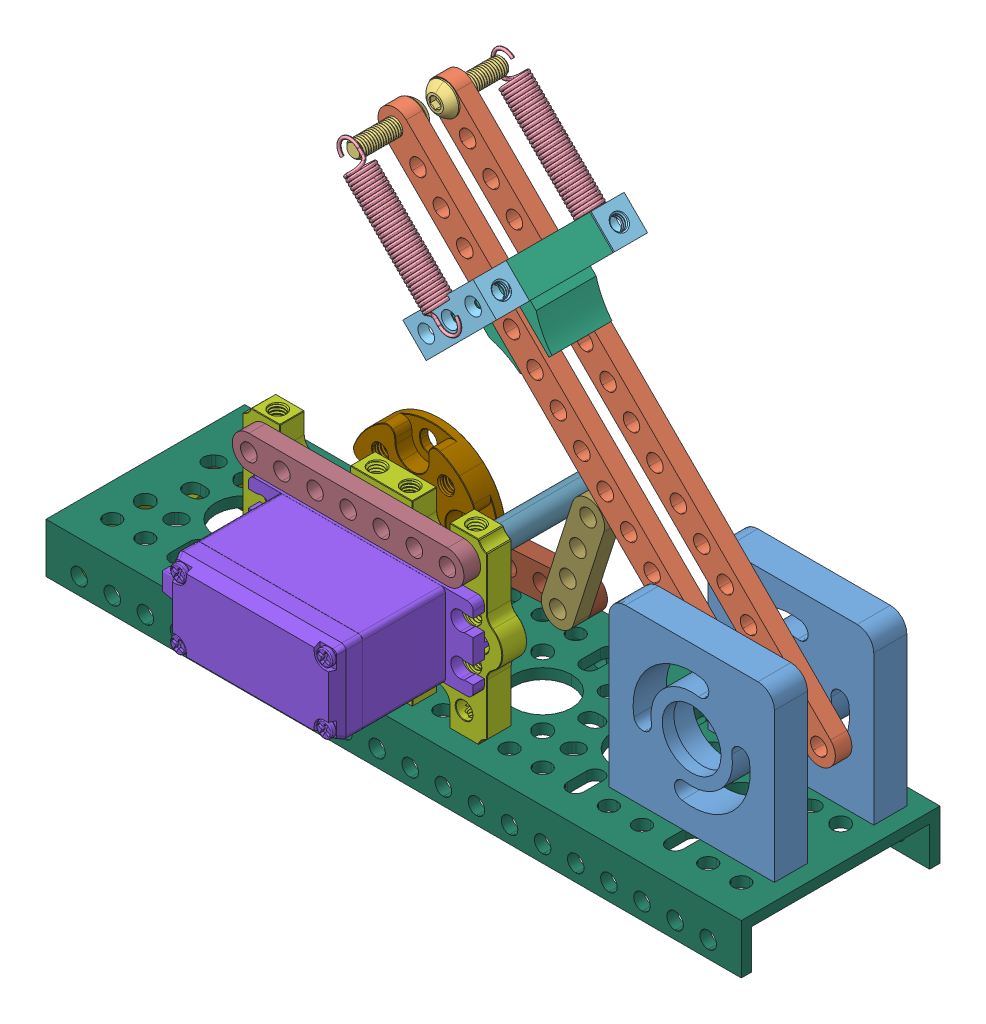
SolidWorks assembly Drone Launcher Assembly League Champs, configuration Default. Lengths in mm.
Overall size (168 121.92 74.59).
40 component instances, 21 part files, 16 mates.
Components (placement in the parent):
- Drone Launcher Assembly-1: Drone Launcher Assembly [Default] at (-2.8899 117.1969 -118.6781) x (-1 0 0) z (0 -1 0) size (105.44 43.78 109.92)
  - Drone Launcher Base-1: Drone Launcher Base [Default] at (9.5832 21.5969 33.0344) size (46.27 8 60.08)
  - Drone Launcher Base-2: Drone Launcher Base [Default] at (9.5832 45.5969 33.0344) size (46.27 8 60.08)
  - 17 hole flat beam.step-1: 17 hole flat beam.step [Default] at (44.1155 29.5969 -5.9724) x (0.707107 0 -0.707107) z (0.707107 0 0.707107) size (136 4 8)
  - 17 hole flat beam.step-2: 17 hole flat beam.step [Default] at (44.1155 41.5969 -5.9724) x (0.707107 0 -0.707107) z (0.707107 0 0.707107) size (136 4 8)
  - 14mm button head screw.step-1: 14mm button head screw.step [Default] at (89.3704 39.3969 -51.2272) x (0.997884 0 -0.065013) z (0 -1 0) size (7.6 7.6 16.21)
  - 14mm button head screw.step-2: 14mm button head screw.step [Default] at (89.3704 35.7969 -51.2272) x (-0.454677 0 -0.890656) z (0 1 0) size (7.6 7.6 16.21)
  - 90404S.stp-1: 90404S.stp [Default] at (77.5883 18.9607 -39.4451) x (0.707107 0 -0.707107) z (-0.707107 0 -0.707107) size (39.64 6.51 6.51)
    - EXTENSION.stp-1: EXTENSION.stp [Default] at origin size (39.64 6.51 6.51)
  - 90404S.stp-3: 90404S.stp [Default] at (77.5883 56.233 -39.4451) x (0.707107 0 -0.707107) z (0.707107 0 0.707107) size (39.64 6.51 6.51)
    - EXTENSION.stp-1: EXTENSION.stp [Default] at origin size (39.64 6.51 6.51)
  - lock nut.step-1: lock nut.step [Default] at (89.3704 18.5946 -51.2272) x (0.258819 0 -0.965926) z (-0.965926 0 -0.258819) (suppressed, hidden)
  - 3 hole square beam.step-1: 3 hole square beam.step [Default] at (60.1493 23.3426 -33.3198) x (0.707107 0 -0.707107) z (0 -1 0) size (8 24.01 8)
  - 3 hole square beam.step-3: 3 hole square beam.step [Default] at (60.1493 51.8511 -33.3198) x (-0.707107 0 0.707107) z (0 1 0) size (8 24.01 8)
  - New Bracket-1: New Bracket [Default] at (68.6346 37.5926 -30.4914) x (0 -1 0) z (-0.707107 0 -0.707107) size (20.5 18 23.2)
  - Spacer For Spring Launcher-1: Spacer For Spring Launcher [Default] at (89.3704 19.3269 -51.2272) x (0.980554 0 0.196247) z (-0.196247 0 0.980554) (suppressed, hidden)
  - Spacer For Spring Launcher-2: Spacer For Spring Launcher [Default] at (89.3704 45.5969 -51.2272) x (0.996904 0 0.078631) z (-0.078631 0 0.996904) (suppressed, hidden)
  - lock nut.step-2: lock nut.step [Default] at (89.3704 56.5991 -51.2272) x (0.707107 0 0.707107) z (-0.707107 0 0.707107) (suppressed, hidden)
- servomounts-2: servomounts [Default] at (-51.5153 70.0218 -135.0382) x (1 0 0) z (0 1 0) size (62.75 6.01 43)
  - 1802-0043-0001 assembly.STEP-1: 1802-0043-0001 assembly.STEP [Default] at origin size (72.97 22.74 55.08)
    - 1802-0043-0001.STEP-1: 1802-0043-0001.STEP [Default] at (-30.9577 -1.7632 15.6407) size (62.75 6.01 43)
    - 2800-0004-0010_90128A207.STEP-1: 2800-0004-0010_90128A207.STEP [Default] at (-69.1779 -7.2859 49.2191) size (7 7 14.01)
    - 2800-0004-0010_90128A207.STEP-2: 2800-0004-0010_90128A207.STEP [Default] at (-62.9116 -10.432 41.1189) size (7 7 14.01)
    - 2800-0004-0010_90128A207.STEP-3: 2800-0004-0010_90128A207.STEP [Default] at (-57.0244 -15.0047 35.4158) size (7 7 14.01)
    - 2800-0004-0010_90128A207.STEP-4: 2800-0004-0010_90128A207.STEP [Default] at (-43.2566 -10.2911 41.7146) size (7 7 14.01)
    - 2801-0004-0008_91166A230.STEP-1: 2801-0004-0008_91166A230.STEP [Default] at (-30.0387 -11.2295 43.9062) size (8 8 1)
    - 2801-0004-0008_91166A230.STEP-2: 2801-0004-0008_91166A230.STEP [Default] at (-23.3551 -8.712 41.3616) size (8 8 1)
    - 2801-0004-0008_91166A230.STEP-3: 2801-0004-0008_91166A230.STEP [Default] at (-15.3435 -8.8342 38.2183) size (8 8 1)
    - 2801-0004-0008_91166A230.STEP-4: 2801-0004-0008_91166A230.STEP [Default] at (-8.3583 -10.7984 34.7791) size (8 8 1)
- servo.step-7: servo.step [Default] at (-82.723 85.7125 -141.7749) x (1 0 0) z (0 0 -1) size (54.3 20 43.9)
- 1910-0025-0816.STEP-2: 1910-0025-0816.STEP [Default] at (-70.1379 71.0056 -167.0522) x (0.752599 -0.65848 0) z (-0.65848 -0.752599 0) size (32 17.1 32)
  - 1910-0025-0816.STEP-1: 1910-0025-0816.STEP [Default] at (-26.5689 7.4772 3.7047) size (32 15.6 32)
  - 2800-0003-0012.STEP-1: 2800-0003-0012.STEP [Default] at (-26.5689 24.5772 3.7047) x (0.895056 0 0.445953) z (0 1 0) size (5.5 5.5 15.01)
- 6 hole flat beam.step-1: 6 hole flat beam.step [Default] at (-80.0672 78.5289 -159.5749) x (0.997783 0.066552 0) z (-0.066552 0.997783 0) size (48 4 8)
- 4 hole flat beam.step-1: 4 hole flat beam.step [Default] at (-56.4621 91.2915 -159.5749) x (0.304122 0.952633 0) z (0.952633 -0.304122 0) size (32 4 8)
- 7 hole flat beam.step-1: 7 hole flat beam.step [Default] at (-84.473 101.6625 -133.2749) x (1 0 0) z (0 -1 0) size (56 4 8)
- 24mm standoff.step-1: 24mm standoff.step [Default] at (-60.473 101.6625 -151.2749) x (0.998632 -0.052296 0) z (0.052296 0.998632 0) size (5.95 24 5.95)
- servo horn-1: servo horn [Default] at (-56.773 85.6625 96.5751) x (-0.852412 -0.522871 0) z (-0.522871 0.852412 0) size (32 33 32) (hidden)
- 6 Hole Low-Side U Channel 168mm.step-1: 6 Hole Low-Side U Channel 168mm.step [Default] at (-156.473 40.1625 -130.7749) x (0 -1 0) z (0 0 1) size (12 168 48)
- dual block.step-1: dual block.step [Default] at (-152.473 40.1625 -152.2749) x (0 -1 0) z (-1 0 0) size (9.5 43 12)
Mates (geometry in assembly coordinates):
- Concentric45: concentric anti-aligned: circle of 1910-0025-0816.STEP-2/1910-0025-0816.STEP-1; cylinder of 6 hole flat beam.step-1 through (-100.0229 77.1978 -163.5749) axis (0 0 -1) radius 2
- Concentric46: concentric anti-aligned: circle of 1910-0025-0816.STEP-2/1910-0025-0816.STEP-1; cylinder of 6 hole flat beam.step-1 through (-84.0583 78.2627 -163.5749) axis (0 0 -1) radius 2
- Coincident63: coincident anti-aligned: plane of 1910-0025-0816.STEP-2/1910-0025-0816.STEP-1 through (-92.573 85.7125 -159.5749) normal (0 0 -1); plane of 6 hole flat beam.step-1 through (-100.0229 77.1978 -159.5749) normal (0 0 1)
- Concentric47: concentric anti-aligned: line of 6 hole flat beam.step-1 through (-60.1116 79.8599 -159.5749) axis (0 0 -1); cylinder of 4 hole flat beam.step-1 through (-60.1116 79.8599 -155.5749) axis (0 0 1) radius 2
- Coincident65: coincident anti-aligned: plane of 6 hole flat beam.step-1 through (-100.0229 77.1978 -159.5749) normal (0 0 1); plane of 4 hole flat beam.step-1 through (-60.1116 79.8599 -159.5749) normal (0 0 -1)
- Concentric48: concentric anti-aligned: circle of servomounts-2/1802-0043-0001 assembly.STEP-1/1802-0043-0001.STEP-1; cylinder of 7 hole flat beam.step-1 through (-108.473 101.6625 -129.2749) axis (0 0 1) radius 2
- Coincident66: coincident anti-aligned: plane of servomounts-2/1802-0043-0001 assembly.STEP-1/1802-0043-0001.STEP-1 through (-82.473 85.6625 -133.2749) normal (0 0 1); plane of 7 hole flat beam.step-1 through (-108.473 101.6625 -133.2749) normal (0 0 -1)
- Concentric49: concentric anti-aligned: cylinder of servomounts-2/1802-0043-0001 assembly.STEP-1/1802-0043-0001.STEP-1 through (-76.473 101.6625 -133.2749) axis (0 0 -1) radius 2.025; cylinder of 7 hole flat beam.step-1 through (-76.473 101.6625 -129.2749) axis (0 0 1) radius 2
- Concentric50: concentric anti-aligned: cylinder of servomounts-2/1802-0043-0001 assembly.STEP-1/1802-0043-0001.STEP-1 through (-60.473 101.6625 -119.6735) axis (0 0 -1) radius 2.025; cylinder of 24mm standoff.step-1 through (-60.473 101.6625 -163.2749) axis (0 0 1) radius 2.975
- Coincident68: coincident anti-aligned: plane of servomounts-2/1802-0043-0001 assembly.STEP-1/1802-0043-0001.STEP-1 through (-82.473 85.6625 -139.2749) normal (0 0 -1); plane of 24mm standoff.step-1 through (-60.473 101.6625 -139.2749) normal (0 0 1)
- Tangent2: tangent anti-aligned: plane of 4 hole flat beam.step-1 through (-63.9221 81.0764 -155.5749) normal (-0.952633 0.304122 0); cylinder of 24mm standoff.step-1 through (-60.473 101.6625 -163.2749) axis (0 0 1) radius 2.975
- Concentric51: concentric anti-aligned: circle of Drone Launcher Assembly-1/Drone Launcher Base-2; cylinder of 6 Hole Low-Side U Channel 168mm.step-1 through (3.527 54.1625 -168.2749) axis (0 1 0) radius 2
- Coincident69: coincident anti-aligned: plane of Drone Launcher Assembly-1/Drone Launcher Base-2 through (7.527 64.1625 -172.2749) normal (0 -1 0); plane of 6 Hole Low-Side U Channel 168mm.step-1 through (11.527 64.1625 -176.2749) normal (0 1 0)
- Coincident70: coincident: plane of 6 Hole Low-Side U Channel 168mm.step-1 through (11.527 61.6625 -130.7749) normal (0 -1 0); plane of dual block.step-1 through (-155.7598 61.6625 -130.7749) normal (0 1 0)
- Coincident71: coincident: plane of 6 Hole Low-Side U Channel 168mm.step-1 through (-166.2965 52.1625 -173.7749) normal (0 0 1); plane of dual block.step-1 through (-155.7598 61.6625 -173.7749) normal (0 0 -1)
- Coincident72: coincident: plane of 6 Hole Low-Side U Channel 168mm.step-1 through (-156.473 40.1625 -130.7749) normal (-1 0 0); plane of dual block.step-1 through (-156.473 38.9125 -152.2749) normal (-1 0 0)
